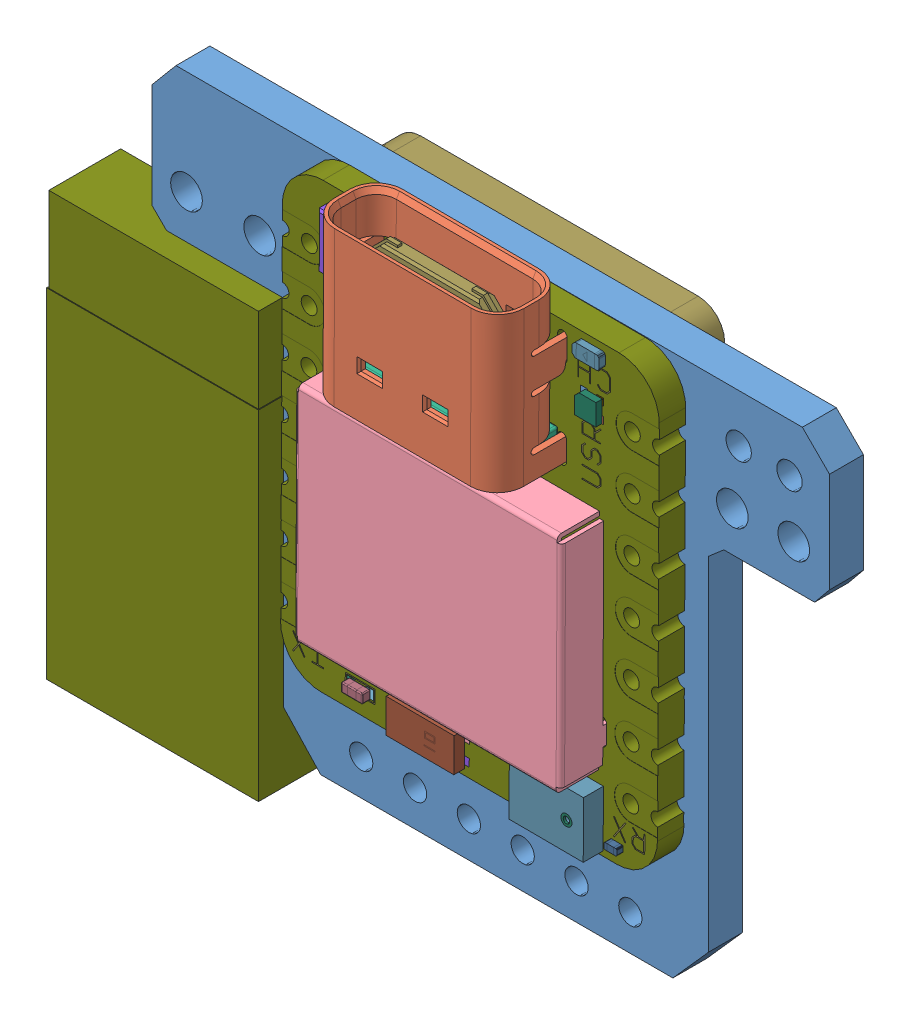
SolidWorks assembly Assem2, configuration Default. Lengths in mm.
Overall size (35.77 28.53 8.56).
97 component instances, 70 part files, 6 mates.
Components (placement in the parent):
- 3D_PCB1_2024-04-28.step-1: 3D_PCB1_2024-04-28.step [Default] at (47.1056 44.0848 -27.5274) size (31.98 25.56 1.6)
  - Board.step-1: Board.step [Default] at origin size (31.98 25.56 1.6)
- XIAO-nRF52840 v15.step-1: XIAO-nRF52840 v15.step [Default] at (-7.7238 14.9491 -25.6774) x (0.004853 0.999988 0) z (0.999988 -0.004853 0) size (22.49 4.48 17.79)
  - USB TYPE C PORT.step-1: USB TYPE C PORT.step [Default] at (4.3161 13.395 -12.1571) x (0 0 -1) z (0 -1 0) size (8.94 7.9 4.2)
    - USB TYPE C PORT (1).step-1: USB TYPE C PORT (1).step [Default] at (-3.0192 1.0963 5.395) size (8.94 7.9 4.2)
      - BOSS-EXTRUDE14_8_.step-1: BOSS-EXTRUDE14_8_.step [Default] at (-3.0192 1.0963 5.395) size (0.6 1 0.3)
      - BOSS-EXTRUDE7_4_.step-1: BOSS-EXTRUDE7_4_.step [Default] at (-3.0192 1.0963 5.395) size (0.3 3.78 0.75)
      - BOSS-EXTRUDE7_3_.step-1: BOSS-EXTRUDE7_3_.step [Default] at (-3.0192 1.0963 5.395) size (0.3 3.78 0.75)
      - BOSS-EXTRUDE14_4_.step-1: BOSS-EXTRUDE14_4_.step [Default] at (-3.0192 1.0963 5.395) size (0.3 1 0.3)
      - BOSS-EXTRUDE14_2_.step-1: BOSS-EXTRUDE14_2_.step [Default] at (-3.0192 1.0963 5.395) size (0.6 1 0.3)
      - BOSS-EXTRUDE14_11_.step-1: BOSS-EXTRUDE14_11_.step [Default] at (-3.0192 1.0963 5.395) size (0.3 1 0.3)
      - BOSS-EXTRUDE7_7_.step-1: BOSS-EXTRUDE7_7_.step [Default] at (-3.0192 1.0963 5.395) size (0.3 3.78 0.75)
      - BOSS-EXTRUDE14_9_.step-1: BOSS-EXTRUDE14_9_.step [Default] at (-3.0192 1.0963 5.395) size (0.3 1 0.3)
      - BOSS-EXTRUDE14_3_.step-1: BOSS-EXTRUDE14_3_.step [Default] at (-3.0192 1.0963 5.395) size (0.3 1 0.3)
      - BOSS-EXTRUDE14_7_.step-1: BOSS-EXTRUDE14_7_.step [Default] at (-3.0192 1.0963 5.395) size (0.6 1 0.3)
      - MIRROR2.step-1: MIRROR2.step [Default] at (-3.0192 1.0963 5.395) size (6.7 4.6 0.7)
      - BOSS-EXTRUDE14_5_.step-1: BOSS-EXTRUDE14_5_.step [Default] at (-3.0192 1.0963 5.395) size (0.3 1 0.3)
      - BOSS-EXTRUDE14_12_.step-1: BOSS-EXTRUDE14_12_.step [Default] at (-3.0192 1.0963 5.395) size (0.3 1 0.3)
      - BOSS-EXTRUDE7_8_.step-1: BOSS-EXTRUDE7_8_.step [Default] at (-3.0192 1.0963 5.395) size (0.3 3.78 0.75)
      - BOSS-EXTRUDE7_1_.step-1: BOSS-EXTRUDE7_1_.step [Default] at (-3.0192 1.0963 5.395) size (0.3 3.78 0.75)
      - BOSS-EXTRUDE14_10_.step-1: BOSS-EXTRUDE14_10_.step [Default] at (-3.0192 1.0963 5.395) size (0.3 1 0.3)
      - BOSS-EXTRUDE7_9_.step-1: BOSS-EXTRUDE7_9_.step [Default] at (-3.0192 1.0963 5.395) size (0.3 3.78 0.75)
      - BOSS-EXTRUDE14_6_.step-1: BOSS-EXTRUDE14_6_.step [Default] at (-3.0192 1.0963 5.395) size (0.6 1 0.3)
      - CHAMFER9.step-1: CHAMFER9.step [Default] at (-3.0192 1.0963 5.395) size (8.94 7.3 4.2)
      - BOSS-EXTRUDE14_1_.step-1: BOSS-EXTRUDE14_1_.step [Default] at (-3.0192 1.0963 5.395) size (0.3 1 0.3)
      - BOSS-EXTRUDE7_6_.step-1: BOSS-EXTRUDE7_6_.step [Default] at (-3.0192 1.0963 5.395) size (0.3 3.78 0.75)
      - BOSS-EXTRUDE7_2_.step-1: BOSS-EXTRUDE7_2_.step [Default] at (-3.0192 1.0963 5.395) size (0.3 3.78 0.75)
      - CUT-EXTRUDE5.step-1: CUT-EXTRUDE5.step [Default] at (-3.0192 1.0963 5.395) size (8.54 2 3.59)
      - BOSS-EXTRUDE7_5_.step-1: BOSS-EXTRUDE7_5_.step [Default] at (-3.0192 1.0963 5.395) size (0.3 3.78 0.75)
  - SKTAAAE010 v1.step-1: SKTAAAE010 v1.step [Default] at (10.4051 1 -11.8268) x (1 0 0) z (0 1 0) size (3.09 1.6 0.73)
    - Body.step-1: Body.step [Default] at (0 0 0.1) size (2.6 1.6 0.63)
    - Pins.step-1: Pins.step [Default] at origin size (3.09 1.19 0.1)
  - PCB (1).step-1: PCB (1).step [Default] at origin size (20.97 1.77 17.79)
    - CAP.step-1: CAP.step [Default] at origin size (0.3 0.3 0.61)
    - ANT1.step-1: ANT1.step [Default] at origin size (1.6 0.5 3.2)
    - Silkscreen.step-1: Silkscreen.step [Default] at origin size (19.14 0.01 16.62)
    - CAP.step-2: CAP.step [Default] at (-1.9064 0 5.2077) size (0.3 0.3 0.61)
    - CAP 3.step-1: CAP 3.step [Default] at origin size (0.44 0.4 1)
    - LED.step-1: LED.step [Default] at origin size (0.64 0.3 1.27)
    - USR.step-1: USR.step [Default] at origin size (1 0.3 1)
    - PCB (1)-0.step-1: PCB (1)-0.step [Default] at origin size (20.97 1.28 17.79)
    - PCB (1)-1.step-1: PCB (1)-1.step [Default] at origin size (0.33 0.01 0.33)
    - PCB (1)-2.step-1: PCB (1)-2.step [Default] at origin size (0.33 0.01 0.33)
    - PCB (1)-3.step-1: PCB (1)-3.step [Default] at origin size (0.33 0.01 0.33)
    - PCB (1)-4.step-1: PCB (1)-4.step [Default] at origin size (0.33 0.01 0.33)
    - PCB (1)-5.step-1: PCB (1)-5.step [Default] at origin size (0.25 0.01 0.07)
    - PCB (1)-6.step-1: PCB (1)-6.step [Default] at origin size (0.37 0.01 0.36)
    - PCB (1)-7.step-1: PCB (1)-7.step [Default] at origin size (0.43 0.01 0.37)
    - PCB (1)-8.step-1: PCB (1)-8.step [Default] at origin size (0.43 0.01 0.37)
    - PCB (1)-9.step-1: PCB (1)-9.step [Default] at origin size (1.29 0.01 0.39)
    - PCB (1)-10.step-1: PCB (1)-10.step [Default] at origin size (0.37 0.01 0.36)
    - PCB (1)-11.step-1: PCB (1)-11.step [Default] at origin size (0.25 0.01 0.14)
    - PCB (1)-12.step-1: PCB (1)-12.step [Default] at origin size (2.11 0.01 1.09)
    - PCB (1)-13.step-1: PCB (1)-13.step [Default] at origin size (2.11 0.01 1.09)
    - PCB (1)-14.step-1: PCB (1)-14.step [Default] at origin size (1.09 0.01 2.11)
    - PCB (1)-15.step-1: PCB (1)-15.step [Default] at origin size (1.09 0.01 2.11)
  - MSM261D3526H1CPM.step-1: MSM261D3526H1CPM.step [Default] at (-0.2514 0 0.4902) size (2.65 0.95 3.5)
    - MSM261D3526H1CPM-16.step-1: MSM261D3526H1CPM-16.step [Default] at origin size (2.65 0.94 3.5)
    - MSM261D3526H1CPM-17.step-1: MSM261D3526H1CPM-17.step [Default] at origin size (0.53 0.1 0.53)
    - MSM261D3526H1CPM-18.step-1: MSM261D3526H1CPM-18.step [Default] at origin size (0.5 0.02 1.03)
    - MSM261D3526H1CPM-19.step-1: MSM261D3526H1CPM-19.step [Default] at origin size (0.62 0.02 1.03)
    - MSM261D3526H1CPM-20.step-1: MSM261D3526H1CPM-20.step [Default] at origin size (0.62 0.02 1.03)
    - MSM261D3526H1CPM-21.step-1: MSM261D3526H1CPM-21.step [Default] at origin size (0.5 0.02 1.03)
    - MSM261D3526H1CPM-22.step-1: MSM261D3526H1CPM-22.step [Default] at origin size (0.62 0.02 1.03)
    - MSM261D3526H1CPM-23.step-1: MSM261D3526H1CPM-23.step [Default] at origin size (0.62 0.02 1.03)
  - Shield.step-1: Shield.step [Default] at (-0.225 0 0) size (10.6 2.7 12.6)
- MAX30102_MH_ET_LIVE_BOARD_v8.step-1: MAX30102_MH_ET_LIVE_BOARD_v8.step [Default] at (-13.7556 17.0103 -27.5274) x (-1 0 0) z (0 0 -1) size (15.6 20.5 2.5)
  - 0603.step-1: 0603.step [Default] at (2.8803 -7.0248 1.3015) size (1.6 0.8 0.45)
    - _X_C4_X_E5_X_F2_X_E0_X_EB_X_FC1.step-1: _X_C4_X_E5_X_F2_X_E0_X_EB_X_FC1.step [Default] at origin size (1 0.8 0.45)
    - _X_C4_X_E5_X_F2_X_E0_X_EB_X_FC2.step-1: _X_C4_X_E5_X_F2_X_E0_X_EB_X_FC2.step [Default] at (-0.5 0 0.225) x (0 1 0) z (-1 0 0) size (0.8 0.45 0.3)
    - _X_C4_X_E5_X_F2_X_E0_X_EB_X_FC2.step-2: _X_C4_X_E5_X_F2_X_E0_X_EB_X_FC2.step [Default] at (0.5 0 0.225) x (0 1 0) z (1 0 0) size (0.8 0.45 0.3)
  - 0805.step-1: 0805.step [Default] at (2.3676 -2.7137 1.3026) size (2 1.2 0.4)
    - _X_C4_X_E5_X_F2_X_E0_X_EB_X_FC1_1.step-1: _X_C4_X_E5_X_F2_X_E0_X_EB_X_FC1_1.step [Default] at origin size (1.2 1.2 0.4)
    - _X_C4_X_E5_X_F2_X_E0_X_EB_X_FC2_1.step-1: _X_C4_X_E5_X_F2_X_E0_X_EB_X_FC2_1.step [Default] at (-0.6 0 0.2) x (0 1 0) z (-1 0 0) size (1.2 0.4 0.4)
    - _X_C4_X_E5_X_F2_X_E0_X_EB_X_FC2_1.step-2: _X_C4_X_E5_X_F2_X_E0_X_EB_X_FC2_1.step [Default] at (0.6 0 0.2) x (0 1 0) z (1 0 0) size (1.2 0.4 0.4)
  - 0805_1.step-1: 0805_1.step [Default] at (2.3676 -4.2137 1.3026) size (2 1.2 0.4)
    - _X_C4_X_E5_X_F2_X_E0_X_EB_X_FC1_1.step-1: _X_C4_X_E5_X_F2_X_E0_X_EB_X_FC1_1.step [Default] at origin size (1.2 1.2 0.4)
    - _X_C4_X_E5_X_F2_X_E0_X_EB_X_FC2_1.step-1: _X_C4_X_E5_X_F2_X_E0_X_EB_X_FC2_1.step [Default] at (-0.6 0 0.2) x (0 1 0) z (-1 0 0) size (1.2 0.4 0.4)
    - _X_C4_X_E5_X_F2_X_E0_X_EB_X_FC2_1.step-2: _X_C4_X_E5_X_F2_X_E0_X_EB_X_FC2_1.step [Default] at (0.6 0 0.2) x (0 1 0) z (1 0 0) size (1.2 0.4 0.4)
  - 0805_2.step-1: 0805_2.step [Default] at (2.3676 -5.7137 1.3026) size (2 1.2 0.4)
    - _X_C4_X_E5_X_F2_X_E0_X_EB_X_FC1_1.step-1: _X_C4_X_E5_X_F2_X_E0_X_EB_X_FC1_1.step [Default] at origin size (1.2 1.2 0.4)
    - _X_C4_X_E5_X_F2_X_E0_X_EB_X_FC2_1.step-1: _X_C4_X_E5_X_F2_X_E0_X_EB_X_FC2_1.step [Default] at (-0.6 0 0.2) x (0 1 0) z (-1 0 0) size (1.2 0.4 0.4)
    - _X_C4_X_E5_X_F2_X_E0_X_EB_X_FC2_1.step-2: _X_C4_X_E5_X_F2_X_E0_X_EB_X_FC2_1.step [Default] at (0.6 0 0.2) x (0 1 0) z (1 0 0) size (1.2 0.4 0.4)
  - SOT-23-6.step-1: SOT-23-6.step [Default] at (2.2999 7.0439 1.3) x (0 -1 0) z (0 0 1) size (2.9 2.4 1)
  - ceramic_cap_0603.step-1: ceramic_cap_0603.step [Default] at (-2.171 -2.6812 1.3021) size (1.6 0.8 0.85)
  - ceramic_cap_0603.step-2: ceramic_cap_0603.step [Default] at (-2.171 3.8188 1.3021) size (1.6 0.8 0.85)
  - ceramic_cap_0603.step-3: ceramic_cap_0603.step [Default] at (-2.171 4.8188 1.3021) size (1.6 0.8 0.85)
  - ceramic_cap_0603.step-4: ceramic_cap_0603.step [Default] at (-2.171 5.8188 1.3021) size (1.6 0.8 0.85)
  - ceramic_cap_0603.step-5: ceramic_cap_0603.step [Default] at (-3.7402 -6.4927 1.3021) x (0 1 0) z (0 0 1) size (1.6 0.8 0.85)
  - ceramic_cap_0603.step-6: ceramic_cap_0603.step [Default] at (-2.1461 6.9108 1.3021) size (1.6 0.8 0.85)
  - ceramic_cap_0603.step-7: ceramic_cap_0603.step [Default] at (1.8992 3.7589 1.3021) size (1.6 0.8 0.85)
  - SOT23-3.step-1: SOT23-3.step [Default] at (-1.3467 -5.9504 1.2808) size (2.84 3.01 1.19)
  - MH_ET_LIVE_BOARD.step-1: MH_ET_LIVE_BOARD.step [Default] at origin size (15.6 20.5 1.3)
  - MH_ET_LIVE_BOARD-0.step-1: MH_ET_LIVE_BOARD-0.step [Default] at origin size (5.7 3.4 1.2)
  - MH_ET_LIVE_BOARD-1.step-1: MH_ET_LIVE_BOARD-1.step [Default] at origin size (1.25 2.76 0.1)
  - MH_ET_LIVE_BOARD-2.step-1: MH_ET_LIVE_BOARD-2.step [Default] at origin size (3.6 2.78 0.1)
- Battery-1: Battery [Default] at (-25.7423 4.3672 -28.2577) size (10 20 3.5)
Mates (geometry in assembly coordinates):
- Distance1: distance = 0 mm: line of 3D_PCB1_2024-04-28.step-1/Board.step-1 through (-28.9445 27.2603 -25.9274) axis (1 0 0); moEndPointRef_w of XIAO-nRF52840 v15.step-1/PCB (1).step-1/PCB (1)-0.step-1
- Coincident3: coincident anti-aligned: plane of 3D_PCB1_2024-04-28.step-1/Board.step-1 through (-14.0227 16.4892 -25.9274) normal (0 0 1); plane of XIAO-nRF52840 v15.step-1/PCB (1).step-1/PCB (1)-0.step-1 through (-13.8264 16.7829 -25.9274) normal (0 0 -1)
- Coincident6: coincident anti-aligned: plane of 3D_PCB1_2024-04-28.step-1/Board.step-1 through (-14.0227 16.4892 -27.5274) normal (0 0 -1); plane of MAX30102_MH_ET_LIVE_BOARD_v8.step-1/MH_ET_LIVE_BOARD.step-1 through (-13.7556 17.0103 -27.5274) normal (0 0 1)
- Coincident8: coincident aligned: line of 3D_PCB1_2024-04-28.step-1/Board.step-1 through (-28.9445 27.2603 -27.5274) axis (1 0 0); line of MAX30102_MH_ET_LIVE_BOARD_v8.step-1/MH_ET_LIVE_BOARD.step-1 through (-20.3056 27.2603 -27.5274) axis (1 0 0)
- Coincident9: coincident anti-aligned: plane of 3D_PCB1_2024-04-28.step-1/Board.step-1 through (-23.8819 3.5897 -27.5274) normal (-1 0 0); plane of Battery-1 through (-23.8819 16.2975 -24.7577) normal (1 0 0)
- Coincident10: coincident anti-aligned: plane of 3D_PCB1_2024-04-28.step-1/Board.step-1 through (-24.6794 20.2975 -27.5274) normal (0 -1 0); plane of Battery-1 through (-25.7423 20.2975 -28.2577) normal (0 1 0)
